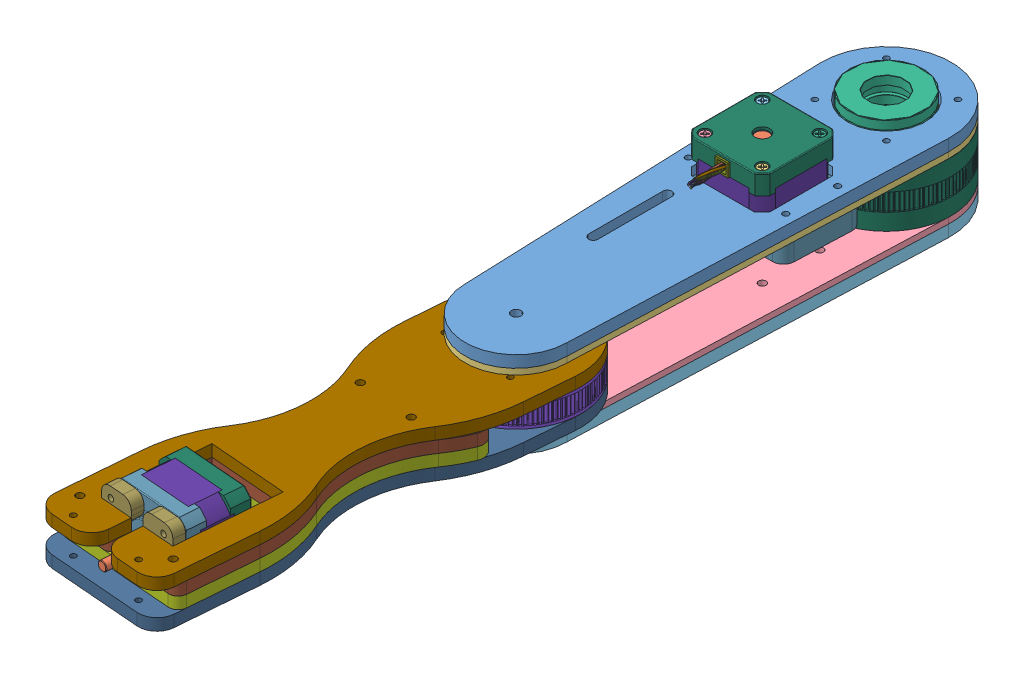
SolidWorks assembly AssemBrasAB, configuration Default. Lengths in mm.
Overall size (139.82 127.63 472.52).
117 component instances, 40 part files, 33 mates.
Components (placement in the parent):
- 03_02_AssemUpperAndLowerArm-1: 03_02_AssemUpperAndLowerArm [Default] at (4.2942 33.9 -117.8774) size (70 11.12 262.5)
  - 03_07_upper&lowerArm-1: 03_07_upper&lowerArm [Default] at (53.4457 141.3704 413.2602) size (70 6.35 262.5)
  - ThrustBallBearingUpper-1: ThrustBallBearingUpper [7806K755] at (53.4457 134.3704 413.2602) x (-0.862828 0 -0.505498) z (-0.505498 0 0.862828) size (40 14 40)
  - upper&lowerbearingFit3mmStepperSide-1: upper&lowerbearingFit3mmStepperSide [Default] at (53.4457 138.1954 313.2602) size (70 3.17 262.5)
- 03_03_AssemUpperAndLowerArm_hex_tete-1: 03_03_AssemUpperAndLowerArm_hex_tete [Défaut] at (77.1604 138.7226 -64.6172) size (70 48.86 262.5)
  - upper&lowerbearingFit3mm-1: upper&lowerbearingFit3mm [Default] at (-19.4206 2.7978 260) size (70 3.17 262.5)
  - 03_07_upper&lowerArm_modif_tete-1: 03_07_upper&lowerArm_modif_tete [Default] at (-19.4206 -3.5522 360) size (70 48.86 262.5)
  - ThrustBallBearingUpper-1: ThrustBallBearingUpper [7806K755] at (-19.4206 9.7978 360) size (40 14 40)
- 03_01_AssemMidArm-1: 03_01_AssemMidArm [Default] at (212.0479 23.0648 -55.3929) x (0.98825 0.030604 0.149751) z (-0.141546 -0.186456 0.972213) size (99.53 77.23 261.45)
  - 7806K755_Thrust Ball Bearing-6: 7806K755_Thrust Ball Bearing [7806K755] at (-95.5251 214.5077 335.8148) x (0.999339 -0.026395 0.025015) z (-0.019643 0.187098 0.982145) size (40 14 40)
  - 7806K755_Thrust Ball Bearing-7: 7806K755_Thrust Ball Bearing [7806K755] at (-96.1234 195.3099 339.46) x (0.408436 -0.182544 -0.894347) z (-0.912274 -0.048784 -0.406666) size (40 14 40)
  - 03_14_midArmUpper-2: 03_14_midArmUpper [Default] at (-95.9237 201.7173 338.2434) x (0.997092 -0.04302 -0.062907) z (0.069795 0.183988 0.980447) size (70 6.35 162)
  - 03_17_customPoulieDenteFinalReworkJoint2-1: 03_17_customPoulieDenteFinalReworkJoint2 [Výchozí] at (-95.8242 204.9088 337.6374) x (-0.644614 0.161957 0.747157) z (0.763896 0.097326 0.637959) size (70 12.55 70)
  - 03_14_BottomArm-2: 03_14_BottomArm [Default] at (-95.535 214.1886 335.8754) x (0.997092 -0.04302 -0.062907) z (0.069795 0.183988 0.980447) size (70 6.35 246.35)
  - 03_13_BottomArm-3: 03_13_BottomArm [Default] at (-96.1181 195.4817 339.4274) x (0.997092 -0.04302 -0.062907) z (0.069795 0.183988 0.980447) size (70 6.35 246.35)
  - 03_04_midArmUpper-3: 03_04_midArmUpper [Default] at (-95.7294 207.953 337.0594) x (0.997092 -0.04302 -0.062907) z (0.069795 0.183988 0.980447) size (70 6.35 162)
  - 03_15_SupportStepper-1: 03_15_SupportStepper [Default] at (-83.0086 238.6246 517.7105) x (0.997092 -0.04302 -0.062907) z (0.069795 0.183988 0.980447) size (57.3 42 6.35)
- 7806K755_Thrust Ball Bearing-1: 7806K755_Thrust Ball Bearing [7806K755] at (57.7399 137.6954 95.3828) x (0.884024 0 -0.467442) z (-0.467442 0 -0.884024) size (40 14 40)
- 7806K755_Thrust Ball Bearing-2: 7806K755_Thrust Ball Bearing [7806K755] at (57.7399 178.9954 95.3828) x (0.977918 0 -0.208988) z (0.208988 0 0.977918) size (40 14 40)
- NEMA17 x 33.step-1: NEMA17 x 33.step [Default] at (57.7399 166.5204 162.3828) size (42 57 60)
  - Copper-2of4.step-1: Copper-2of4.step [Défaut] at (0 28 0) x (0 1 0) z (0 0 1) size (2.77 3.05 24)
  - Frontplate.step-1: Frontplate.step [Défaut] at (0 10.5 0) size (42 12.5 42)
  - Backplate.step-1: Backplate.step [Défaut] at (0 33 0) size (42 10.5 42)
  - Connenctor.step-1: Connenctor.step [Défaut] at (0 24.5 22) size (7 7 7)
  - Housing.step-1: Housing.step [Défaut] at (0 7.5 0) size (42 17 42)
  - Bearing dummy.step-1: Bearing dummy.step [Défaut] at (0 4 0) size (22 7 22)
  - Bearing dummy 01.step-1: Bearing dummy 01.step [Défaut] at (0 28 0) size (22 7 22)
  - Core.step-1: Core.step [Défaut] at origin size (30 55.5 30)
  - M3x25-Screw.step-1: M3x25-Screw.step [Default] at (15.5 30.6 15.5) x (1 0 0) z (0 1 0) size (5.5 5.5 27)
  - M3x25-Screw004.step-1: M3x25-Screw004.step [Default] at (-15.5 30.6 15.5) x (1 0 0) z (0 1 0) size (5.5 5.5 27)
  - M3x25-Screw005.step-1: M3x25-Screw005.step [Default] at (-15.5 30.6 -15.5) x (1 0 0) z (0 1 0) size (5.5 5.5 27)
  - M3x25-Screw006.step-1: M3x25-Screw006.step [Default] at (15.5 30.6 -15.5) x (1 0 0) z (0 1 0) size (5.5 5.5 27)
  - Cable-1of4.step-1: Cable-1of4.step [Défaut] at (0 28 0) size (3.44 3.69 21)
  - Copper-1of4.step-1: Copper-1of4.step [Défaut] at (0 28 0) size (2.77 3.05 24)
  - Cable-2of4.step-1: Cable-2of4.step [Défaut] at (0 28 0) x (0 1 0) z (0 0 1) size (3.44 3.69 21)
  - Copper-4of4.step-1: Copper-4of4.step [Défaut] at (0 28 0) x (0 -1 0) z (0 0 1) size (2.77 3.05 24)
  - Cable-3of4.step-1: Cable-3of4.step [Défaut] at (0 28 0) x (-1 0 0) z (0 0 1) size (3.44 3.69 21)
  - Copper-3of4.step-1: Copper-3of4.step [Défaut] at (0 28 0) x (-1 0 0) z (0 0 1) size (2.77 3.05 24)
  - Cable-4of4.step-1: Cable-4of4.step [Défaut] at (0 28 0) x (0 -1 0) z (0 0 1) size (3.44 3.69 21)
- 03_016_supportStepper-1: 03_016_supportStepper [Default] at (57.7399 162.5204 162.3828) x (0 0 -1) z (1 0 0) size (42 9.57 66.17)
- 03_10_customPoulieDenteFinalReworkJoint1-1: 03_10_customPoulieDenteFinalReworkJoint1 [Výchozí] at (57.7399 158.3454 95.3828) x (0.707107 0 -0.707107) z (0.707107 0 0.707107) size (70 27.3 70)
- T5 Pulley-1: T5 Pulley [Predeterminado] at (57.7399 147.6204 162.3828) x (0 1 0) z (-0.646857 0 0.762611) size (14.8 16 16)
- Bearing Subassy, GT2 Idler Pulley, Configurable-1: Bearing Subassy, GT2 Idler Pulley, Configurable [5 mm Bore] at (57.7399 143.0204 162.3828) size (9 3 9)
  - Bearing Outer Ring, GT2 Idler Pulley, Configurable-1: Bearing Outer Ring, GT2 Idler Pulley, Configurable [5 mm Bore] at origin size (9 3 9)
  - Bearing Inner Ring, GT2 Idler Pulley, Configurable-1: Bearing Inner Ring, GT2 Idler Pulley, Configurable [5 mm Bore] x (0.926062 0 -0.377371) z (0.377371 0 0.926062) size (6 3 6)
  - Bearing Seal, GT2 Idler Pulley, Configurable-1: Bearing Seal, GT2 Idler Pulley, Configurable [5 mm Bore] at (0 1.25 0) size (8 0.5 8)
  - Bearing Seal, GT2 Idler Pulley, Configurable-2: Bearing Seal, GT2 Idler Pulley, Configurable [5 mm Bore] at (0 -1.25 0) x (1 0 0) z (0 0 -1) size (8 0.5 8)
  - Bearing Ball, GT2 Idler Pulley, Configurable-1: Bearing Ball, GT2 Idler Pulley, Configurable [1.4 mm] at (-2.4745 0 -2.4753) x (-0.715461 0 0.698652) z (-0.698652 0 -0.715461) size (1.4 1.4 1.4)
  - Bearing Ball, GT2 Idler Pulley, Configurable-2: Bearing Ball, GT2 Idler Pulley, Configurable [1.4 mm] at (-0.9053 0 -3.3809) x (-0.968934 0 0.24732) z (-0.24732 0 -0.968934) size (1.4 1.4 1.4)
  - Bearing Ball, GT2 Idler Pulley, Configurable-3: Bearing Ball, GT2 Idler Pulley, Configurable [1.4 mm] at (0.9064 0 -3.3806) x (-0.962781 0 -0.270282) z (0.270282 0 -0.962781) size (1.4 1.4 1.4)
  - Bearing Ball, GT2 Idler Pulley, Configurable-4: Bearing Ball, GT2 Idler Pulley, Configurable [1.4 mm] at (2.4753 0 -2.4745) x (-0.698652 0 -0.715461) z (0.715461 0 -0.698652) size (1.4 1.4 1.4)
  - Bearing Ball, GT2 Idler Pulley, Configurable-5: Bearing Ball, GT2 Idler Pulley, Configurable [1.4 mm] at (3.3809 0 -0.9053) x (-0.24732 0 -0.968934) z (0.968934 0 -0.24732) size (1.4 1.4 1.4)
  - Bearing Ball, GT2 Idler Pulley, Configurable-6: Bearing Ball, GT2 Idler Pulley, Configurable [1.4 mm] at (3.3806 0 0.9064) x (0.270282 0 -0.962781) z (0.962781 0 0.270282) size (1.4 1.4 1.4)
  - Bearing Ball, GT2 Idler Pulley, Configurable-7: Bearing Ball, GT2 Idler Pulley, Configurable [1.4 mm] at (2.4745 0 2.4753) x (0.715461 0 -0.698652) z (0.698652 0 0.715461) size (1.4 1.4 1.4)
  - Bearing Ball, GT2 Idler Pulley, Configurable-8: Bearing Ball, GT2 Idler Pulley, Configurable [1.4 mm] at (0.9053 0 3.3809) x (0.968934 0 -0.24732) z (0.24732 0 0.968934) size (1.4 1.4 1.4)
  - Bearing Ball, GT2 Idler Pulley, Configurable-9: Bearing Ball, GT2 Idler Pulley, Configurable [1.4 mm] at (-0.9064 0 3.3806) x (0.962781 0 0.270282) z (-0.270282 0 0.962781) size (1.4 1.4 1.4)
  - Bearing Ball, GT2 Idler Pulley, Configurable-10: Bearing Ball, GT2 Idler Pulley, Configurable [1.4 mm] at (-2.4753 0 2.4745) x (0.698652 0 0.715461) z (-0.715461 0 0.698652) size (1.4 1.4 1.4)
  - Bearing Ball, GT2 Idler Pulley, Configurable-11: Bearing Ball, GT2 Idler Pulley, Configurable [1.4 mm] at (-3.3809 0 0.9053) x (0.24732 0 0.968934) z (-0.968934 0 0.24732) size (1.4 1.4 1.4)
  - Bearing Ball, GT2 Idler Pulley, Configurable-12: Bearing Ball, GT2 Idler Pulley, Configurable [1.4 mm] at (-3.3806 0 -0.9064) x (-0.270282 0 0.962781) z (-0.962781 0 -0.270282) size (1.4 1.4 1.4)
- NEMA17 x 33.step-3: NEMA17 x 33.step [Default] at (42.9716 158.3204 478.438) x (-0.996761 0 -0.080415) z (0 -1 0) size (42 57 60)
  - Copper-2of4.step-1: Copper-2of4.step [Défaut] at (0 28 0) x (0 1 0) z (0 0 1) size (2.77 3.05 24)
  - Frontplate.step-1: Frontplate.step [Défaut] at (0 10.5 0) size (42 12.5 42)
  - Backplate.step-1: Backplate.step [Défaut] at (0 33 0) size (42 10.5 42)
  - Connenctor.step-1: Connenctor.step [Défaut] at (0 24.5 22) size (7 7 7)
  - Housing.step-1: Housing.step [Défaut] at (0 7.5 0) size (42 17 42)
  - Bearing dummy.step-1: Bearing dummy.step [Défaut] at (0 4 0) size (22 7 22)
  - Bearing dummy 01.step-1: Bearing dummy 01.step [Défaut] at (0 28 0) size (22 7 22)
  - Core.step-1: Core.step [Défaut] at origin size (30 55.5 30)
  - M3x25-Screw.step-1: M3x25-Screw.step [Default] at (15.5 30.6 15.5) x (1 0 0) z (0 1 0) size (5.5 5.5 27)
  - M3x25-Screw004.step-1: M3x25-Screw004.step [Default] at (-15.5 30.6 15.5) x (1 0 0) z (0 1 0) size (5.5 5.5 27)
  - M3x25-Screw005.step-1: M3x25-Screw005.step [Default] at (-15.5 30.6 -15.5) x (1 0 0) z (0 1 0) size (5.5 5.5 27)
  - M3x25-Screw006.step-1: M3x25-Screw006.step [Default] at (15.5 30.6 -15.5) x (1 0 0) z (0 1 0) size (5.5 5.5 27)
  - Cable-1of4.step-1: Cable-1of4.step [Défaut] at (0 28 0) size (3.44 3.69 21)
  - Copper-1of4.step-1: Copper-1of4.step [Défaut] at (0 28 0) size (2.77 3.05 24)
  - Cable-2of4.step-1: Cable-2of4.step [Défaut] at (0 28 0) x (0 1 0) z (0 0 1) size (3.44 3.69 21)
  - Copper-4of4.step-1: Copper-4of4.step [Défaut] at (0 28 0) x (0 -1 0) z (0 0 1) size (2.77 3.05 24)
  - Cable-3of4.step-1: Cable-3of4.step [Défaut] at (0 28 0) x (-1 0 0) z (0 0 1) size (3.44 3.69 21)
  - Copper-3of4.step-1: Copper-3of4.step [Défaut] at (0 28 0) x (-1 0 0) z (0 0 1) size (2.77 3.05 24)
  - Cable-4of4.step-1: Cable-4of4.step [Défaut] at (0 28 0) x (0 -1 0) z (0 0 1) size (3.44 3.69 21)
- pulleyColonne-1: pulleyColonne [Default] at (42.7399 171.1954 226.1729) x (-0.741677 0 -0.670758) z (-0.670758 0 0.741677) size (20 9 20)
- pulleyColonne-2: pulleyColonne [Default] at (42.7399 144.6954 226.1729) size (20 9 20)
- GT2 Idler Pulley, Configurable-1: GT2 Idler Pulley, Configurable [20T W6 B5 Without T] at (42.7399 157.9454 226.1729) size (25.32 8.5 25.32)
  - Body, GT2 Idler Pulley, Configurable-1: Body, GT2 Idler Pulley, Configurable [20T W6 B5 Without T] x (-0.63029 0 -0.77636) z (0.77636 0 -0.63029) size (18 8.5 18)
  - Bearing Subassy, GT2 Idler Pulley, Configurable-1: Bearing Subassy, GT2 Idler Pulley, Configurable [5 mm Bore] at (0 2.75 0) x (0.63029 0 0.77636) z (-0.77636 0 0.63029) size (9 3 9)
    - Bearing Outer Ring, GT2 Idler Pulley, Configurable-1: Bearing Outer Ring, GT2 Idler Pulley, Configurable [5 mm Bore] at origin size (9 3 9)
    - Bearing Inner Ring, GT2 Idler Pulley, Configurable-1: Bearing Inner Ring, GT2 Idler Pulley, Configurable [5 mm Bore] x (0.926062 0 -0.377371) z (0.377371 0 0.926062) size (6 3 6)
    - Bearing Seal, GT2 Idler Pulley, Configurable-1: Bearing Seal, GT2 Idler Pulley, Configurable [5 mm Bore] at (0 1.25 0) size (8 0.5 8)
    - Bearing Seal, GT2 Idler Pulley, Configurable-2: Bearing Seal, GT2 Idler Pulley, Configurable [5 mm Bore] at (0 -1.25 0) x (1 0 0) z (0 0 -1) size (8 0.5 8)
    - Bearing Ball, GT2 Idler Pulley, Configurable-1: Bearing Ball, GT2 Idler Pulley, Configurable [1.4 mm] at (-2.4745 0 -2.4753) x (-0.715461 0 0.698652) z (-0.698652 0 -0.715461) size (1.4 1.4 1.4)
    - Bearing Ball, GT2 Idler Pulley, Configurable-2: Bearing Ball, GT2 Idler Pulley, Configurable [1.4 mm] at (-0.9053 0 -3.3809) x (-0.968934 0 0.24732) z (-0.24732 0 -0.968934) size (1.4 1.4 1.4)
    - Bearing Ball, GT2 Idler Pulley, Configurable-3: Bearing Ball, GT2 Idler Pulley, Configurable [1.4 mm] at (0.9064 0 -3.3806) x (-0.962781 0 -0.270282) z (0.270282 0 -0.962781) size (1.4 1.4 1.4)
    - Bearing Ball, GT2 Idler Pulley, Configurable-4: Bearing Ball, GT2 Idler Pulley, Configurable [1.4 mm] at (2.4753 0 -2.4745) x (-0.698652 0 -0.715461) z (0.715461 0 -0.698652) size (1.4 1.4 1.4)
    - Bearing Ball, GT2 Idler Pulley, Configurable-5: Bearing Ball, GT2 Idler Pulley, Configurable [1.4 mm] at (3.3809 0 -0.9053) x (-0.24732 0 -0.968934) z (0.968934 0 -0.24732) size (1.4 1.4 1.4)
    - Bearing Ball, GT2 Idler Pulley, Configurable-6: Bearing Ball, GT2 Idler Pulley, Configurable [1.4 mm] at (3.3806 0 0.9064) x (0.270282 0 -0.962781) z (0.962781 0 0.270282) size (1.4 1.4 1.4)
    - Bearing Ball, GT2 Idler Pulley, Configurable-7: Bearing Ball, GT2 Idler Pulley, Configurable [1.4 mm] at (2.4745 0 2.4753) x (0.715461 0 -0.698652) z (0.698652 0 0.715461) size (1.4 1.4 1.4)
    - Bearing Ball, GT2 Idler Pulley, Configurable-8: Bearing Ball, GT2 Idler Pulley, Configurable [1.4 mm] at (0.9053 0 3.3809) x (0.968934 0 -0.24732) z (0.24732 0 0.968934) size (1.4 1.4 1.4)
    - Bearing Ball, GT2 Idler Pulley, Configurable-9: Bearing Ball, GT2 Idler Pulley, Configurable [1.4 mm] at (-0.9064 0 3.3806) x (0.962781 0 0.270282) z (-0.270282 0 0.962781) size (1.4 1.4 1.4)
    - Bearing Ball, GT2 Idler Pulley, Configurable-10: Bearing Ball, GT2 Idler Pulley, Configurable [1.4 mm] at (-2.4753 0 2.4745) x (0.698652 0 0.715461) z (-0.715461 0 0.698652) size (1.4 1.4 1.4)
    - Bearing Ball, GT2 Idler Pulley, Configurable-11: Bearing Ball, GT2 Idler Pulley, Configurable [1.4 mm] at (-3.3809 0 0.9053) x (0.24732 0 0.968934) z (-0.968934 0 0.24732) size (1.4 1.4 1.4)
    - Bearing Ball, GT2 Idler Pulley, Configurable-12: Bearing Ball, GT2 Idler Pulley, Configurable [1.4 mm] at (-3.3806 0 -0.9064) x (-0.270282 0 0.962781) z (-0.962781 0 -0.270282) size (1.4 1.4 1.4)
  - Bearing Subassy, GT2 Idler Pulley, Configurable-2: Bearing Subassy, GT2 Idler Pulley, Configurable [5 mm Bore] at (0 -2.75 0) x (0.63029 0 0.77636) z (0.77636 0 -0.63029) size (9 3 9)
    - Bearing Outer Ring, GT2 Idler Pulley, Configurable-1: Bearing Outer Ring, GT2 Idler Pulley, Configurable [5 mm Bore] at origin size (9 3 9)
    - Bearing Inner Ring, GT2 Idler Pulley, Configurable-1: Bearing Inner Ring, GT2 Idler Pulley, Configurable [5 mm Bore] x (0.926062 0 -0.377371) z (0.377371 0 0.926062) size (6 3 6)
    - Bearing Seal, GT2 Idler Pulley, Configurable-1: Bearing Seal, GT2 Idler Pulley, Configurable [5 mm Bore] at (0 1.25 0) size (8 0.5 8)
    - Bearing Seal, GT2 Idler Pulley, Configurable-2: Bearing Seal, GT2 Idler Pulley, Configurable [5 mm Bore] at (0 -1.25 0) x (1 0 0) z (0 0 -1) size (8 0.5 8)
    - Bearing Ball, GT2 Idler Pulley, Configurable-1: Bearing Ball, GT2 Idler Pulley, Configurable [1.4 mm] at (-2.4745 0 -2.4753) x (-0.715461 0 0.698652) z (-0.698652 0 -0.715461) size (1.4 1.4 1.4)
    - Bearing Ball, GT2 Idler Pulley, Configurable-2: Bearing Ball, GT2 Idler Pulley, Configurable [1.4 mm] at (-0.9053 0 -3.3809) x (-0.968934 0 0.24732) z (-0.24732 0 -0.968934) size (1.4 1.4 1.4)
    - Bearing Ball, GT2 Idler Pulley, Configurable-3: Bearing Ball, GT2 Idler Pulley, Configurable [1.4 mm] at (0.9064 0 -3.3806) x (-0.962781 0 -0.270282) z (0.270282 0 -0.962781) size (1.4 1.4 1.4)
    - Bearing Ball, GT2 Idler Pulley, Configurable-4: Bearing Ball, GT2 Idler Pulley, Configurable [1.4 mm] at (2.4753 0 -2.4745) x (-0.698652 0 -0.715461) z (0.715461 0 -0.698652) size (1.4 1.4 1.4)
    - Bearing Ball, GT2 Idler Pulley, Configurable-5: Bearing Ball, GT2 Idler Pulley, Configurable [1.4 mm] at (3.3809 0 -0.9053) x (-0.24732 0 -0.968934) z (0.968934 0 -0.24732) size (1.4 1.4 1.4)
    - Bearing Ball, GT2 Idler Pulley, Configurable-6: Bearing Ball, GT2 Idler Pulley, Configurable [1.4 mm] at (3.3806 0 0.9064) x (0.270282 0 -0.962781) z (0.962781 0 0.270282) size (1.4 1.4 1.4)
    - Bearing Ball, GT2 Idler Pulley, Configurable-7: Bearing Ball, GT2 Idler Pulley, Configurable [1.4 mm] at (2.4745 0 2.4753) x (0.715461 0 -0.698652) z (0.698652 0 0.715461) size (1.4 1.4 1.4)
    - Bearing Ball, GT2 Idler Pulley, Configurable-8: Bearing Ball, GT2 Idler Pulley, Configurable [1.4 mm] at (0.9053 0 3.3809) x (0.968934 0 -0.24732) z (0.24732 0 0.968934) size (1.4 1.4 1.4)
    - Bearing Ball, GT2 Idler Pulley, Configurable-9: Bearing Ball, GT2 Idler Pulley, Configurable [1.4 mm] at (-0.9064 0 3.3806) x (0.962781 0 0.270282) z (-0.270282 0 0.962781) size (1.4 1.4 1.4)
    - Bearing Ball, GT2 Idler Pulley, Configurable-10: Bearing Ball, GT2 Idler Pulley, Configurable [1.4 mm] at (-2.4753 0 2.4745) x (0.698652 0 0.715461) z (-0.715461 0 0.698652) size (1.4 1.4 1.4)
    - Bearing Ball, GT2 Idler Pulley, Configurable-11: Bearing Ball, GT2 Idler Pulley, Configurable [1.4 mm] at (-3.3809 0 0.9053) x (0.24732 0 0.968934) z (-0.968934 0 0.24732) size (1.4 1.4 1.4)
    - Bearing Ball, GT2 Idler Pulley, Configurable-12: Bearing Ball, GT2 Idler Pulley, Configurable [1.4 mm] at (-3.3806 0 -0.9064) x (-0.270282 0 0.962781) z (-0.962781 0 -0.270282) size (1.4 1.4 1.4)
Mates (geometry in assembly coordinates):
- Concentric3: concentric anti-aligned: circle of 03_02_AssemUpperAndLowerArm-1/ThrustBallBearingUpper-1; circle of 03_03_AssemUpperAndLowerArm_hex_tete-1/ThrustBallBearingUpper-1
- Concentric5: concentric anti-aligned: circle of 03_03_AssemUpperAndLowerArm_hex_tete-1/ThrustBallBearingUpper-1; circle of 03_01_AssemMidArm-1/7806K755_Thrust Ball Bearing-7
- Concentric7: concentric aligned: circle of 03_03_AssemUpperAndLowerArm_hex_tete-1/03_07_upper&lowerArm_modif_tete-1; circle of 7806K755_Thrust Ball Bearing-1
- Concentric8: concentric anti-aligned: circle of 03_02_AssemUpperAndLowerArm-1/03_07_upper&lowerArm-1; circle of 7806K755_Thrust Ball Bearing-2
- Distance1: distance = 14.1 mm anti-aligned: plane of 03_01_AssemMidArm-1/03_17_customPoulieDenteFinalReworkJoint2-1 through (57.7399 161.1704 295.3828) normal (0 1 0); plane of 03_02_AssemUpperAndLowerArm-1/03_07_upper&lowerArm-1 through (57.7399 175.2704 295.3828) normal (0 -1 0)
- Distance2: distance = 14.1 mm anti-aligned: plane of 03_01_AssemMidArm-1/03_17_customPoulieDenteFinalReworkJoint2-1 through (57.7399 155.6204 295.3828) normal (0 -1 0); plane of 03_03_AssemUpperAndLowerArm_hex_tete-1/03_07_upper&lowerArm_modif_tete-1 through (57.7399 141.5204 295.3828) normal (0 1 0)
- Coincident1: coincident anti-aligned: plane of 03_02_AssemUpperAndLowerArm-1/upper&lowerbearingFit3mm-1 through (57.7399 172.0954 195.3828) normal (0 -1 0); plane of 03_10_customPoulieDenteFinalReworkJoint1-1 through (57.7399 171.9954 95.3828) normal (0 1 0)
- Concentric9: concentric anti-aligned: circle of 03_02_AssemUpperAndLowerArm-1/03_07_upper&lowerArm-1; circle of 03_10_customPoulieDenteFinalReworkJoint1-1
- Concentric10: concentric anti-aligned: circle of 03_02_AssemUpperAndLowerArm-1/03_07_upper&lowerArm-1; circle of 03_10_customPoulieDenteFinalReworkJoint1-1
- Parallel1: parallel aligned: plane of 03_02_AssemUpperAndLowerArm-1/03_07_upper&lowerArm-1 through (57.7399 181.6204 295.3828) normal (0 1 0); plane of NEMA17 x 33.step-1/Backplate.step-1 through (57.7399 199.5204 162.3828) normal (0 1 0)
- Coincident4: coincident aligned: plane of 03_01_AssemMidArm-1/03_17_customPoulieDenteFinalReworkJoint2-1 through (57.7399 153.6204 295.3828) normal (0 1 0); plane of T5 Pulley-1 through (52.4016 153.6204 157.8548) normal (0 1 0)
- Concentric11: concentric aligned: cylinder of NEMA17 x 33.step-1/Core.step-1 through (57.7399 142.8204 162.3828) axis (0 1 0) radius 2.5; cylinder of T5 Pulley-1 through (57.7399 144.4204 162.3828) axis (0 1 0) radius 2.5
- Coincident5: coincident aligned: plane of 03_02_AssemUpperAndLowerArm-1/03_07_upper&lowerArm-1 through (57.7399 175.2704 295.3828) normal (1 0 0); plane of NEMA17 x 33.step-1 through (57.7399 166.5204 162.3828) normal (1 0 0)
- Distance4: distance = 1 mm: plane of NEMA17 x 33.step-1/Core.step-1 through (57.7399 142.5204 162.3828) normal (0 -1 0); line of 03_03_AssemUpperAndLowerArm_hex_tete-1/upper&lowerbearingFit3mm-1 through (85.2399 141.5204 295.3828) axis (0.037597 0 -0.999293)
- Coincident6: coincident anti-aligned: plane of 03_03_AssemUpperAndLowerArm_hex_tete-1/03_07_upper&lowerArm_modif_tete-1 through (57.7399 141.5204 295.3828) normal (0 1 0); plane of Bearing Subassy, GT2 Idler Pulley, Configurable-1/Bearing Outer Ring, GT2 Idler Pulley, Configurable-1 through (57.7399 141.5204 162.3828) normal (0 -1 0)
- Concentric13: concentric anti-aligned: cylinder of NEMA17 x 33.step-1/Frontplate.step-1 through (57.7399 166.5204 162.3828) axis (0 -1 0) radius 11; circle of 03_016_supportStepper-1
- Parallel2: parallel aligned: plane of NEMA17 x 33.step-1/Frontplate.step-1 through (74.7104 177.0204 183.3828) normal (0 0 1); plane of 03_016_supportStepper-1 through (89.4729 166.5204 182.8726) normal (0 0 1)
- Coincident7: coincident anti-aligned: plane of NEMA17 x 33.step-1/Frontplate.step-1 through (57.7399 166.5204 162.3828) normal (0 -1 0); plane of 03_016_supportStepper-1 through (57.7399 166.5204 162.3828) normal (0 1 0)
- Coincident8: coincident anti-aligned: plane of 03_02_AssemUpperAndLowerArm-1/03_07_upper&lowerArm-1 through (40.7618 175.2704 141.3828) normal (0 0 1); plane of NEMA17 x 33.step-1/Backplate.step-1 through (40.7693 199.5204 141.3828) normal (0 0 -1)
- Concentric15: concentric aligned: cylinder of 03_03_AssemUpperAndLowerArm_hex_tete-1/upper&lowerbearingFit3mm-1 through (57.7399 141.5204 162.3828) axis (0 1 0) radius 4.425; circle of Bearing Subassy, GT2 Idler Pulley, Configurable-1/Bearing Outer Ring, GT2 Idler Pulley, Configurable-1
- Coincident9: coincident anti-aligned: plane of 7806K755_Thrust Ball Bearing-2 through (47.8238 171.9954 97.5019) normal (0 -1 0); plane of 03_10_customPoulieDenteFinalReworkJoint1-1 through (57.7399 171.9954 95.3828) normal (0 1 0)
- Concentric16: concentric anti-aligned: circle of 03_03_AssemUpperAndLowerArm_hex_tete-1/03_07_upper&lowerArm_modif_tete-1; circle of 03_10_customPoulieDenteFinalReworkJoint1-1
- Coincident10: coincident anti-aligned: plane of 03_03_AssemUpperAndLowerArm_hex_tete-1/upper&lowerbearingFit3mm-1 through (57.7399 144.6954 195.3828) normal (0 1 0); plane of 03_10_customPoulieDenteFinalReworkJoint1-1 through (57.7399 144.6954 95.3828) normal (0 -1 0)
- Coincident11: coincident anti-aligned: plane of 7806K755_Thrust Ball Bearing-1 through (48.7759 144.6954 100.1227) normal (0 1 0); plane of 03_10_customPoulieDenteFinalReworkJoint1-1 through (57.7399 144.6954 95.3828) normal (0 -1 0)
- Coincident20: coincident anti-aligned: plane of 03_01_AssemMidArm-1/03_15_SupportStepper-1 through (42.9716 158.3204 478.438) normal (0.080415 0 -0.996761); plane of NEMA17 x 33.step-3/Frontplate.step-1 through (42.9716 158.3204 478.438) normal (-0.080415 0 0.996761)
- Concentric19: concentric aligned: cylinder of 03_01_AssemMidArm-1/03_15_SupportStepper-1 through (42.9716 158.3204 478.438) axis (-0.080415 0 0.996761) radius 11; cylinder of NEMA17 x 33.step-3/Frontplate.step-1 through (42.9716 158.3204 478.438) axis (-0.080415 0 0.996761) radius 11
- Coincident21: coincident anti-aligned: plane of 03_01_AssemMidArm-1/03_14_BottomArm-2 through (78.6719 164.6704 297.0715) normal (-0.996761 0 -0.080415); plane of NEMA17 x 33.step-3/Frontplate.step-1 through (64.7479 141.3499 469.6608) normal (0.996761 0 0.080415)
- Coincident22: coincident anti-aligned: plane of pulleyColonne-2 through (42.7399 153.6954 226.1729) normal (0 1 0); plane of GT2 Idler Pulley, Configurable-1/Body, GT2 Idler Pulley, Configurable-1 through (39.9036 153.6954 222.6792) normal (0 -1 0)
- Concentric20: concentric aligned: circle of pulleyColonne-2; circle of GT2 Idler Pulley, Configurable-1/Body, GT2 Idler Pulley, Configurable-1
- Coincident23: coincident anti-aligned: plane of pulleyColonne-1 through (42.7399 162.1954 226.1729) normal (0 -1 0); plane of GT2 Idler Pulley, Configurable-1/Body, GT2 Idler Pulley, Configurable-1 through (37.0673 162.1954 219.1856) normal (0 1 0)
- Concentric21: concentric anti-aligned: circle of pulleyColonne-1; circle of GT2 Idler Pulley, Configurable-1/Body, GT2 Idler Pulley, Configurable-1
- Coincident24: coincident anti-aligned: plane of 03_03_AssemUpperAndLowerArm_hex_tete-1/upper&lowerbearingFit3mm-1 through (57.7399 144.6954 195.3828) normal (0 1 0); plane of pulleyColonne-2 through (42.7399 144.6954 226.1729) normal (0 -1 0)
- Slot1: slot anti-aligned: cylinder of pulleyColonne-2 through (42.7399 153.6954 226.1729) axis (0 -1 0) radius 3; plane of 03_03_AssemUpperAndLowerArm_hex_tete-1/03_07_upper&lowerArm_modif_tete-1 through (46.7399 135.1704 238.6828) normal (-1 0 0); cylinder of 03_03_AssemUpperAndLowerArm_hex_tete-1/03_07_upper&lowerArm_modif_tete-1 through (42.7399 135.1704 198.6828) axis (0 1 0) radius 4
